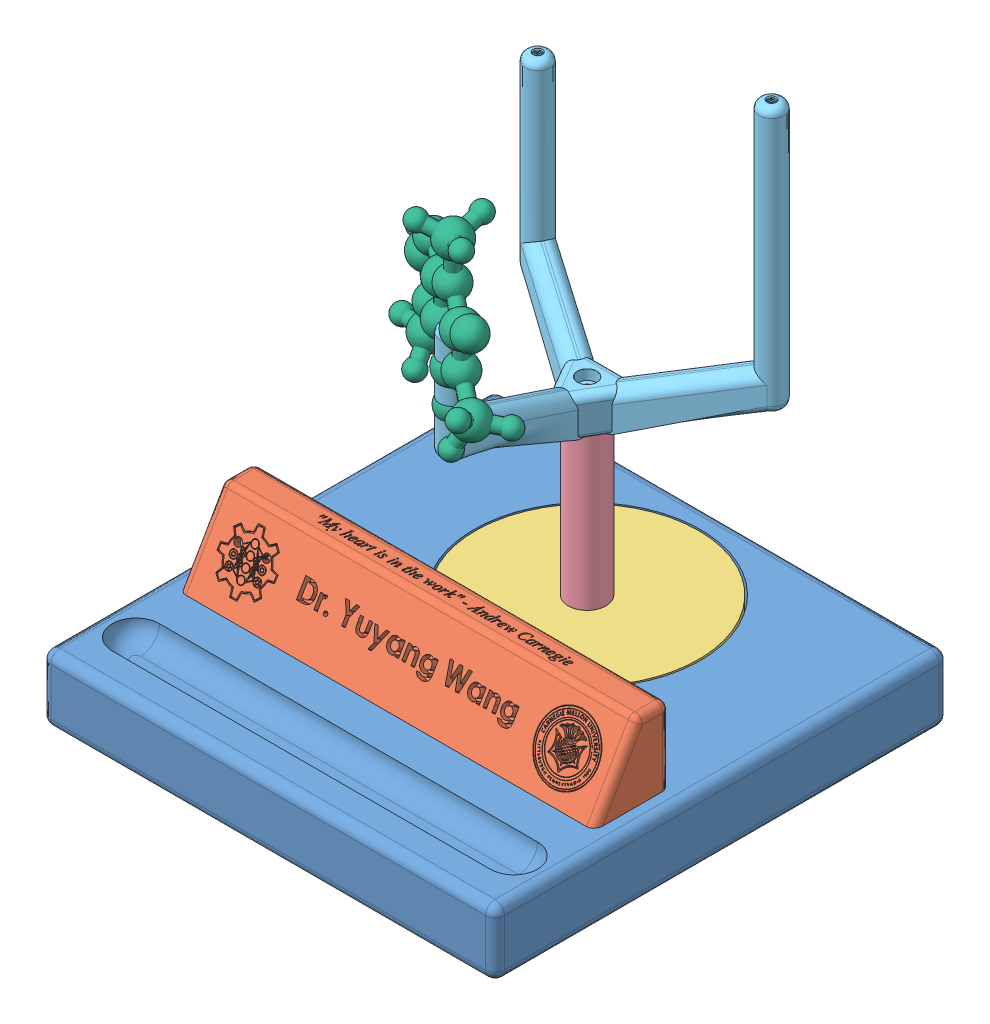
SolidWorks assembly PenHolderV1, configuration Default. Lengths in mm.
Overall size (152.4 174.62 152.4).
6 component instances, 6 part files, 8 mates.
Components (placement in the parent):
- Base-1: Base [9246K573] at origin size (152.4 22.23 152.4)
- NamePlate-1: NamePlate [Default] at (0 11.1125 23.8125) size (139.7 25.4 25.4)
- Mount-1: Mount [Default] at (0 -1.5875 -30.9563) size (74.93 12.7 74.93)
- Stand-1: Stand [Default] at (0 11.1125 -30.9563) size (12.7 50.8 12.7)
- ModelMounts-1: ModelMounts [Default] at (0 61.9125 -30.9563) size (86.95 101.91 76.42)
- CaffeineMolecule-1: CaffeineMolecule [Default] at (-0.0949 110.2019 -0.5905) x (-0.785345 -0.346374 -0.513086) z (-0.546944 0 0.837169) size (72.4 61.97 23.63)
Mates (geometry in assembly coordinates):
- Coincident3: coincident anti-aligned: plane of Base-1 through (-76.2 11.1125 76.2) normal (0 1 0); plane of NamePlate-1 through (0 11.1125 23.8125) normal (0 -1 0)
- Distance11: distance = 12.7 mm: line of NamePlate-1 through (-67.31 11.1125 36.5125) axis (1 0 0); line of Base-1 through (63.5 11.1125 49.2125) axis (-1 0 0)
- Concentric2: concentric anti-aligned: circle of Base-1; circle of Mount-1
- Concentric3: concentric aligned: circle of Mount-1; circle of Stand-1
- Coincident5: coincident aligned: plane of Mount-1 through (0 11.1125 -30.9563) normal (0 1 0); circle of Stand-1
- Concentric4: concentric aligned: circle of Stand-1; circle of ModelMounts-1
- Coincident6: coincident anti-aligned: plane of Stand-1 through (0 61.9125 -30.9563) normal (0 1 0); plane of ModelMounts-1 through (0 61.9125 -30.9563) normal (0 -1 0)
- Concentric5: concentric aligned: cylinder of ModelMounts-1; cylinder of CaffeineMolecule-1 through (0 106.0087 14.4028) axis (0 1 0) radius 1.8
